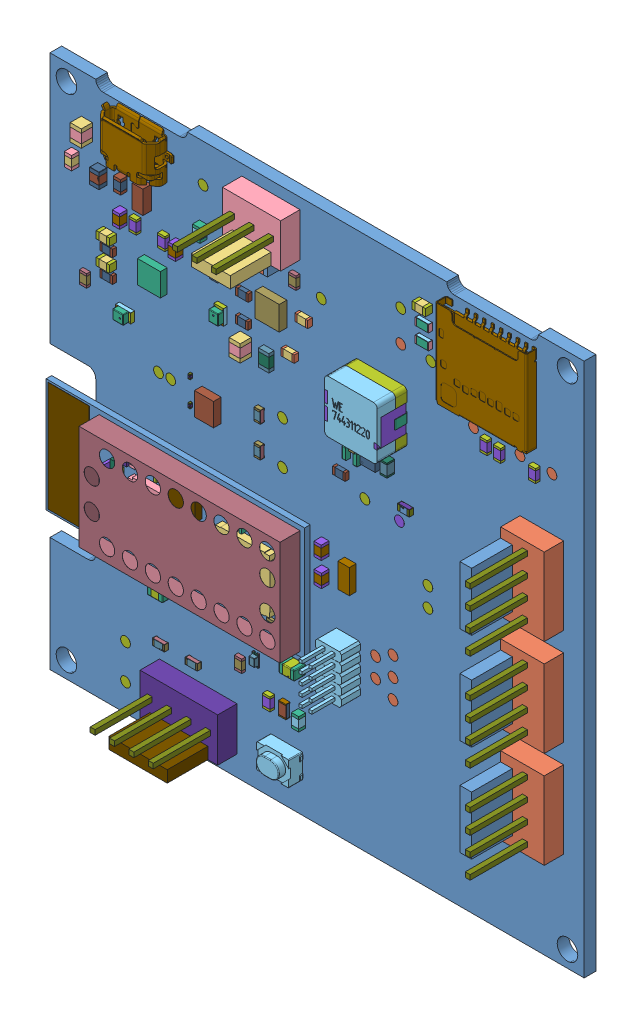
SolidWorks assembly IoTracking_PCB_new, configuration Default. Lengths in mm.
Overall size (70 70 13.59).
656 component instances, 214 part files, 0 mates.
Components (placement in the parent):
- IoTracking_PCB_new.step-1: IoTracking_PCB_new.step [Default] at origin size (70.02 70.02 13.59)
  - Board.step-1: Board.step [Default] at origin size (70 70 1.53)
    - Open CASCADE STEP translator 6.8 1.1.1.step-1: Open CASCADE STEP translator 6.8 1.1.1.step [Default] at (0 0 -1.5342) size (70 70 1.53)
  - TP8.step-1: TP8.step [Default] at origin size (1.27 1.27 0.02)
    - 6125959248.step-1: 6125959248.step [Default] at (42.672 22.86 -0.015) x (-1 0 0) z (0 0 1) size (1.27 1.27 0.02)
      - Cylinder.step-1: Cylinder.step [Default] at origin size (1.27 1.27 0.02)
  - C3.step-1: C3.step [Default] at origin size (0.95 1.75 0.95)
    - 6125953728.step-1: 6125953728.step [Default] at (3.302 59.817 0) size (0.95 0.95 0.95)
      - Extruded.step-1: Extruded.step [Default] at origin size (0.95 0.95 0.95)
    - 6125953568.step-1: 6125953568.step [Default] at (3.302 59.142 0) size (0.95 0.4 0.95)
      - Extruded-0.step-1: Extruded-0.step [Default] at origin size (0.95 0.4 0.95)
    - 6125953568.step-2: 6125953568.step [Default] at (3.302 60.492 0) size (0.95 0.4 0.95)
      - Extruded-0.step-1: Extruded-0.step [Default] at origin size (0.95 0.4 0.95)
  - B1.step-1: B1.step [Default] at origin size (4.6 3.2 2.5)
    - PTS810_CK_Switch.step-1: PTS810_CK_Switch.step [Default] at (30.9881 5.5881 0) x (1 0 0) z (0 -1 0) size (4.6 2.5 3.2)
  - C9.step-1: C9.step [Default] at origin size (2.01 1.25 1.52)
    - Cap_AVX_0805YA103FAT2A_eec.step-1: Cap_AVX_0805YA103FAT2A_eec.step [Default] at (32.512 16.764 0) x (1 0 0) z (0 0 1) size (2.01 1.25 1.52)
      - Terminals.step-1: Terminals.step [Default] at origin size (2.01 1.25 1.52)
      - Electrode.step-1: Electrode.step [Default] at origin size (1.01 1.25 1.52)
      - AVX.step-1: AVX.step [Default] at origin size (0.37 0.13 0)
  - X1.step-1: X1.step [Default] at origin size (1.5 3.2 0.9)
    - 6125955888.step-1: 6125955888.step [Default] at (39.37 30.48 0) size (1.5 3.2 0.9)
      - Extruded-1.step-1: Extruded-1.step [Default] at origin size (1.5 3.2 0.9)
  - U_Buck1.step-1: U_Buck1.step [Default] at origin size (2 2 0.8)
    - 5928732880.step-1: 5928732880.step [Default] at (42.418 45.466 0) x (0 1 0) z (1 0 0) size (2 0.8 2)
  - U_Accel1.step-1: U_Accel1.step [Default] at origin size (2.5 3 1)
    - 6125958608.step-1: 6125958608.step [Default] at (21.1836 40.64 0) size (2.5 3 1)
      - Extruded-2.step-1: Extruded-2.step [Default] at origin size (2.5 3 1)
  - U4.step-1: U4.step [Default] at origin size (3.15 3.15 1)
    - 6127423232.step-1: 6127423232.step [Default] at (29.464 55.88 0) size (3.15 3.15 1)
      - Extruded-3.step-1: Extruded-3.step [Default] at origin size (3.15 3.15 1)
  - U3.step-1: U3.step [Default] at origin size (33.86 14.91 3.4)
    - SAMW25.step-1: SAMW25.step [Default] at (60.2291 61.0334 0) x (1 0 0) z (0 0 1) size (33.86 14.91 3.4)
      - wifimodule.step-1: wifimodule.step [Default] at (-37.621 -27.6339 0) x (-1 0 0) z (0 0 1) size (26.34 13.71 2.64)
      - wifimodule_2.step-1: wifimodule_2.step [Default] at (-37.621 -27.6339 0) x (-1 0 0) z (0 0 1) size (0.33 0.95 0.33)
      - wifimodule_3.step-1: wifimodule_3.step [Default] at (-37.621 -27.6339 0) x (-1 0 0) z (0 0 1) size (0.95 0.33 0.33)
      - wifimodule_4.step-1: wifimodule_4.step [Default] at (-37.621 -27.6339 0) x (-1 0 0) z (0 0 1) size (0.33 0.95 0.33)
      - wifimodule_5.step-1: wifimodule_5.step [Default] at (-37.621 -27.6339 0) x (-1 0 0) z (0 0 1) size (0.33 0.95 0.33)
      - wifimodule_6.step-1: wifimodule_6.step [Default] at (-37.621 -27.6339 0) x (-1 0 0) z (0 0 1) size (0.33 0.95 0.33)
      - wifimodule_7.step-1: wifimodule_7.step [Default] at (-37.621 -27.6339 0) x (-1 0 0) z (0 0 1) size (3.7 2.1 0.6)
      - wifimodule_8.step-1: wifimodule_8.step [Default] at (-37.621 -27.6339 0) x (-1 0 0) z (0 0 1) size (0.33 0.95 0.33)
      - wifimodule_9.step-1: wifimodule_9.step [Default] at (-37.621 -27.6339 0) x (-1 0 0) z (0 0 1) size (0.5 1 0.03)
      - wifimodule_10.step-1: wifimodule_10.step [Default] at (-37.621 -27.6339 0) x (-1 0 0) z (0 0 1) size (0.5 1 0.03)
      - wifimodule_11.step-1: wifimodule_11.step [Default] at (-37.621 -27.6339 0) x (-1 0 0) z (0 0 1) size (0.5 1 0.03)
      - wifimodule_12.step-1: wifimodule_12.step [Default] at (-37.621 -27.6339 0) x (-1 0 0) z (0 0 1) size (0.5 1 0.03)
      - wifimodule_13.step-1: wifimodule_13.step [Default] at (-37.621 -27.6339 0) x (-1 0 0) z (0 0 1) size (0.5 1 0.03)
      - wifimodule_14.step-1: wifimodule_14.step [Default] at (-37.621 -27.6339 0) x (-1 0 0) z (0 0 1) size (0.5 1 0.03)
      - wifimodule_15.step-1: wifimodule_15.step [Default] at (-37.621 -27.6339 0) x (-1 0 0) z (0 0 1) size (0.5 1 0.03)
      - wifimodule_16.step-1: wifimodule_16.step [Default] at (-37.621 -27.6339 0) x (-1 0 0) z (0 0 1) size (0.5 1 0.03)
      - wifimodule_17.step-1: wifimodule_17.step [Default] at (-37.621 -27.6339 0) x (-1 0 0) z (0 0 1) size (0.5 1 0.03)
      - wifimodule_18.step-1: wifimodule_18.step [Default] at (-37.621 -27.6339 0) x (-1 0 0) z (0 0 1) size (0.5 1 0.03)
      - wifimodule_19.step-1: wifimodule_19.step [Default] at (-37.621 -27.6339 0) x (-1 0 0) z (0 0 1) size (0.5 1 0.03)
      - wifimodule_20.step-1: wifimodule_20.step [Default] at (-37.621 -27.6339 0) x (-1 0 0) z (0 0 1) size (0.5 1 0.03)
      - wifimodule_21.step-1: wifimodule_21.step [Default] at (-37.621 -27.6339 0) x (-1 0 0) z (0 0 1) size (0.5 1 0.03)
      - wifimodule_22.step-1: wifimodule_22.step [Default] at (-37.621 -27.6339 0) x (-1 0 0) z (0 0 1) size (0.5 1 0.03)
      - wifimodule_23.step-1: wifimodule_23.step [Default] at (-37.621 -27.6339 0) x (-1 0 0) z (0 0 1) size (0.5 1 0.03)
      - wifimodule_24.step-1: wifimodule_24.step [Default] at (-37.621 -27.6339 0) x (-1 0 0) z (0 0 1) size (0.95 0.33 0.33)
      - wifimodule_25.step-1: wifimodule_25.step [Default] at (-37.621 -27.6339 0) x (-1 0 0) z (0 0 1) size (0.95 0.33 0.33)
      - wifimodule_26.step-1: wifimodule_26.step [Default] at (-37.621 -27.6339 0) x (-1 0 0) z (0 0 1) size (0.95 0.33 0.33)
      - wifimodule_27.step-1: wifimodule_27.step [Default] at (-37.621 -27.6339 0) x (-1 0 0) z (0 0 1) size (0.33 0.95 0.33)
      - wifimodule_28.step-1: wifimodule_28.step [Default] at (-37.621 -27.6339 0) x (-1 0 0) z (0 0 1) size (0.95 0.33 0.33)
      - wifimodule_29.step-1: wifimodule_29.step [Default] at (-37.621 -27.6339 0) x (-1 0 0) z (0 0 1) size (0.33 0.95 0.33)
      - wifimodule_30.step-1: wifimodule_30.step [Default] at (-37.621 -27.6339 0) x (-1 0 0) z (0 0 1) size (0.95 0.33 0.33)
      - wifimodule_31.step-1: wifimodule_31.step [Default] at (-37.621 -27.6339 0) x (-1 0 0) z (0 0 1) size (0.33 0.95 0.33)
      - wifimodule_32.step-1: wifimodule_32.step [Default] at (-37.621 -27.6339 0) x (-1 0 0) z (0 0 1) size (0.33 0.74 1)
      - wifimodule_33.step-1: wifimodule_33.step [Default] at (-37.621 -27.6339 0) x (-1 0 0) z (0 0 1) size (0.74 0.33 1)
      - wifimodule_34.step-1: wifimodule_34.step [Default] at (-37.621 -27.6339 0) x (-1 0 0) z (0 0 1) size (2.68 1.78 1.04)
      - wifimodule_35.step-1: wifimodule_35.step [Default] at (-37.621 -27.6339 0) x (-1 0 0) z (0 0 1) size (1.56 1.02 0.66)
      - wifimodule_36.step-1: wifimodule_36.step [Default] at (-37.621 -27.6339 0) x (-1 0 0) z (0 0 1) size (0.91 2.06 0.41)
      - wifimodule_37.step-1: wifimodule_37.step [Default] at (-37.621 -27.6339 0) x (-1 0 0) z (0 0 1) size (2.06 0.91 0.41)
      - wifimodule_38.step-1: wifimodule_38.step [Default] at (-37.621 -27.6339 0) x (-1 0 0) z (0 0 1) size (2.06 0.91 0.41)
      - wifimodule_39.step-1: wifimodule_39.step [Default] at (-37.621 -27.6339 0) x (-1 0 0) z (0 0 1) size (0.91 2.06 0.41)
      - wifimodule_40.step-1: wifimodule_40.step [Default] at (-37.621 -27.6339 0) x (-1 0 0) z (0 0 1) size (0.33 0.74 1)
      - wifimodule_41.step-1: wifimodule_41.step [Default] at (-37.621 -27.6339 0) x (-1 0 0) z (0 0 1) size (0.33 0.74 1)
      - wifimodule_42.step-1: wifimodule_42.step [Default] at (-37.621 -27.6339 0) x (-1 0 0) z (0 0 1) size (0.33 0.74 1)
      - wifimodule_43.step-1: wifimodule_43.step [Default] at (-37.621 -27.6339 0) x (-1 0 0) z (0 0 1) size (0.33 0.74 1)
      - wifimodule_44.step-1: wifimodule_44.step [Default] at (-37.621 -27.6339 0) x (-1 0 0) z (0 0 1) size (0.33 0.74 1)
      - wifimodule_45.step-1: wifimodule_45.step [Default] at (-37.621 -27.6339 0) x (-1 0 0) z (0 0 1) size (0.74 0.33 1)
      - wifimodule_46.step-1: wifimodule_46.step [Default] at (-37.621 -27.6339 0) x (-1 0 0) z (0 0 1) size (0.74 0.33 1)
      - wifimodule_47.step-1: wifimodule_47.step [Default] at (-37.621 -27.6339 0) x (-1 0 0) z (0 0 1) size (0.33 0.74 1)
      - wifimodule_48.step-1: wifimodule_48.step [Default] at (-37.621 -27.6339 0) x (-1 0 0) z (0 0 1) size (0.33 0.74 1)
      - wifimodule_49.step-1: wifimodule_49.step [Default] at (-37.621 -27.6339 0) x (-1 0 0) z (0 0 1) size (0.33 0.74 1)
      - wifimodule_50.step-1: wifimodule_50.step [Default] at (-37.621 -27.6339 0) x (-1 0 0) z (0 0 1) size (0.74 0.33 1)
      - wifimodule_51.step-1: wifimodule_51.step [Default] at (-37.621 -27.6339 0) x (-1 0 0) z (0 0 1) size (0.74 0.33 1)
      - wifimodule_52.step-1: wifimodule_52.step [Default] at (-37.621 -27.6339 0) x (-1 0 0) z (0 0 1) size (0.74 0.33 1)
      - wifimodule_53.step-1: wifimodule_53.step [Default] at (-37.621 -27.6339 0) x (-1 0 0) z (0 0 1) size (0.74 0.33 1)
      - wifimodule_54.step-1: wifimodule_54.step [Default] at (-37.621 -27.6339 0) x (-1 0 0) z (0 0 1) size (0.74 0.33 1)
      - wifimodule_55.step-1: wifimodule_55.step [Default] at (-37.621 -27.6339 0) x (-1 0 0) z (0 0 1) size (0.33 0.74 1)
      - wifimodule_56.step-1: wifimodule_56.step [Default] at (-37.621 -27.6339 0) x (-1 0 0) z (0 0 1) size (0.74 0.33 1)
      - wifimodule_57.step-1: wifimodule_57.step [Default] at (-37.621 -27.6339 0) x (-1 0 0) z (0 0 1) size (0.42 1.12 0.33)
      - wifimodule_58.step-1: wifimodule_58.step [Default] at (-37.621 -27.6339 0) x (-1 0 0) z (0 0 1) size (0.5 1 0.03)
      - wifimodule_59.step-1: wifimodule_59.step [Default] at (-37.621 -27.6339 0) x (-1 0 0) z (0 0 1) size (0.42 1.12 0.33)
      - wifimodule_60.step-1: wifimodule_60.step [Default] at (-37.621 -27.6339 0) x (-1 0 0) z (0 0 1) size (3.66 4.34 0.91)
      - wifimodule_61.step-1: wifimodule_61.step [Default] at (-37.621 -27.6339 0) x (-1 0 0) z (0 0 1) size (0.5 1 0.03)
      - wifimodule_62.step-1: wifimodule_62.step [Default] at (-37.621 -27.6339 0) x (-1 0 0) z (0 0 1) size (0.5 1 0.03)
      - wifimodule_63.step-1: wifimodule_63.step [Default] at (-37.621 -27.6339 0) x (-1 0 0) z (0 0 1) size (0.5 1 0.03)
      - wifimodule_64.step-1: wifimodule_64.step [Default] at (-37.621 -27.6339 0) x (-1 0 0) z (0 0 1) size (0.5 1 0.03)
      - wifimodule_65.step-1: wifimodule_65.step [Default] at (-37.621 -27.6339 0) x (-1 0 0) z (0 0 1) size (1 0.5 0.03)
      - wifimodule_66.step-1: wifimodule_66.step [Default] at (-37.621 -27.6339 0) x (-1 0 0) z (0 0 1) size (1 0.5 0.03)
      - wifimodule_67.step-1: wifimodule_67.step [Default] at (-37.621 -27.6339 0) x (-1 0 0) z (0 0 1) size (1 0.5 0.03)
      - wifimodule_68.step-1: wifimodule_68.step [Default] at (-37.621 -27.6339 0) x (-1 0 0) z (0 0 1) size (1 0.5 0.03)
      - wifimodule_69.step-1: wifimodule_69.step [Default] at (-37.621 -27.6339 0) x (-1 0 0) z (0 0 1) size (1 0.5 0.03)
      - wifimodule_70.step-1: wifimodule_70.step [Default] at (-37.621 -27.6339 0) x (-1 0 0) z (0 0 1) size (1 0.5 0.03)
      - wifimodule_71.step-1: wifimodule_71.step [Default] at (-37.621 -27.6339 0) x (-1 0 0) z (0 0 1) size (1 0.5 0.03)
      - wifimodule_72.step-1: wifimodule_72.step [Default] at (-37.621 -27.6339 0) x (-1 0 0) z (0 0 1) size (0.5 1 0.03)
      - wifimodule_73.step-1: wifimodule_73.step [Default] at (-37.621 -27.6339 0) x (-1 0 0) z (0 0 1) size (0.5 1 0.03)
      - wifimodule_74.step-1: wifimodule_74.step [Default] at (-37.621 -27.6339 0) x (-1 0 0) z (0 0 1) size (0.5 1 0.03)
      - wifimodule_75.step-1: wifimodule_75.step [Default] at (-37.621 -27.6339 0) x (-1 0 0) z (0 0 1) size (0.5 1 0.03)
      - wifimodule_76.step-1: wifimodule_76.step [Default] at (-37.621 -27.6339 0) x (-1 0 0) z (0 0 1) size (0.5 1 0.03)
      - wifimodule_77.step-1: wifimodule_77.step [Default] at (-37.621 -27.6339 0) x (-1 0 0) z (0 0 1) size (0.5 1 0.03)
      - wifimodule_78.step-1: wifimodule_78.step [Default] at (-37.621 -27.6339 0) x (-1 0 0) z (0 0 1) size (0.5 1 0.03)
      - wifimodule_79.step-1: wifimodule_79.step [Default] at (-37.621 -27.6339 0) x (-1 0 0) z (0 0 1) size (0.5 1 0.03)
      - wifimodule_80.step-1: wifimodule_80.step [Default] at (-37.621 -27.6339 0) x (-1 0 0) z (0 0 1) size (0.95 0.33 0.33)
      - wifimodule_81.step-1: wifimodule_81.step [Default] at (-37.621 -27.6339 0) x (-1 0 0) z (0 0 1) size (0.95 0.33 0.33)
      - wifimodule_82.step-1: wifimodule_82.step [Default] at (-37.621 -27.6339 0) x (-1 0 0) z (0 0 1) size (0.33 0.95 0.33)
      - wifimodule_83.step-1: wifimodule_83.step [Default] at (-37.621 -27.6339 0) x (-1 0 0) z (0 0 1) size (0.33 0.95 0.33)
      - wifimodule_84.step-1: wifimodule_84.step [Default] at (-37.621 -27.6339 0) x (-1 0 0) z (0 0 1) size (1.12 0.42 0.33)
      - wifimodule_85.step-1: wifimodule_85.step [Default] at (-37.621 -27.6339 0) x (-1 0 0) z (0 0 1) size (0.95 0.33 0.33)
      - wifimodule_86.step-1: wifimodule_86.step [Default] at (-37.621 -27.6339 0) x (-1 0 0) z (0 0 1) size (0.42 1.12 0.33)
      - wifimodule_87.step-1: wifimodule_87.step [Default] at (-37.621 -27.6339 0) x (-1 0 0) z (0 0 1) size (0.95 0.33 0.33)
      - wifimodule_88.step-1: wifimodule_88.step [Default] at (-37.621 -27.6339 0) x (-1 0 0) z (0 0 1) size (1 0.5 0.03)
      - wifimodule_89.step-1: wifimodule_89.step [Default] at (-37.621 -27.6339 0) x (-1 0 0) z (0 0 1) size (0.5 1 0.03)
      - wifimodule_90.step-1: wifimodule_90.step [Default] at (-37.621 -27.6339 0) x (-1 0 0) z (0 0 1) size (0.5 1 0.03)
      - wifimodule_91.step-1: wifimodule_91.step [Default] at (-37.621 -27.6339 0) x (-1 0 0) z (0 0 1) size (0.5 1 0.03)
      - wifimodule_92.step-1: wifimodule_92.step [Default] at (-37.621 -27.6339 0) x (-1 0 0) z (0 0 1) size (1 0.5 0.03)
      - wifimodule_93.step-1: wifimodule_93.step [Default] at (-37.621 -27.6339 0) x (-1 0 0) z (0 0 1) size (0.5 1 0.03)
      - wifimodule_94.step-1: wifimodule_94.step [Default] at (-37.621 -27.6339 0) x (-1 0 0) z (0 0 1) size (0.5 1 0.03)
      - wifimodule_95.step-1: wifimodule_95.step [Default] at (-37.621 -27.6339 0) x (-1 0 0) z (0 0 1) size (0.5 1 0.03)
      - wifimodule_96.step-1: wifimodule_96.step [Default] at (-37.621 -27.6339 0) x (-1 0 0) z (0 0 1) size (0.5 1 0.03)
      - wifimodule_97.step-1: wifimodule_97.step [Default] at (-37.621 -27.6339 0) x (-1 0 0) z (0 0 1) size (0.5 1 0.03)
      - wifimodule_98.step-1: wifimodule_98.step [Default] at (-37.621 -27.6339 0) x (-1 0 0) z (0 0 1) size (1 0.5 0.03)
      - wifimodule_99.step-1: wifimodule_99.step [Default] at (-37.621 -27.6339 0) x (-1 0 0) z (0 0 1) size (1 0.5 0.03)
      - wifimodule_100.step-1: wifimodule_100.step [Default] at (-37.621 -27.6339 0) x (-1 0 0) z (0 0 1) size (0.5 1 0.03)
      - wifimodule_101.step-1: wifimodule_101.step [Default] at (-37.621 -27.6339 0) x (-1 0 0) z (0 0 1) size (0.5 1 0.03)
      - wifimodule_102.step-1: wifimodule_102.step [Default] at (-37.621 -27.6339 0) x (-1 0 0) z (0 0 1) size (0.5 1 0.03)
      - wifimodule_103.step-1: wifimodule_103.step [Default] at (-37.621 -27.6339 0) x (-1 0 0) z (0 0 1) size (0.5 1 0.03)
      - wifimodule_104.step-1: wifimodule_104.step [Default] at (-37.621 -27.6339 0) x (-1 0 0) z (0 0 1) size (0.33 0.95 0.33)
      - wifimodule_105.step-1: wifimodule_105.step [Default] at (-37.621 -27.6339 0) x (-1 0 0) z (0 0 1) size (0.33 0.95 0.33)
      - wifimodule_106.step-1: wifimodule_106.step [Default] at (-37.621 -27.6339 0) x (-1 0 0) z (0 0 1) size (0.33 0.95 0.33)
      - wifimodule_107.step-1: wifimodule_107.step [Default] at (-37.621 -27.6339 0) x (-1 0 0) z (0 0 1) size (0.33 0.95 0.33)
      - wifimodule_108.step-1: wifimodule_108.step [Default] at (-37.621 -27.6339 0) x (-1 0 0) z (0 0 1) size (0.95 0.33 0.33)
      - wifimodule_109.step-1: wifimodule_109.step [Default] at (-37.621 -27.6339 0) x (-1 0 0) z (0 0 1) size (0.33 0.95 0.33)
      - wifimodule_110.step-1: wifimodule_110.step [Default] at (-37.621 -27.6339 0) x (-1 0 0) z (0 0 1) size (0.33 0.95 0.33)
      - wifimodule_111.step-1: wifimodule_111.step [Default] at (-37.621 -27.6339 0) x (-1 0 0) z (0 0 1) size (0.74 0.33 1)
      - wifimodule_112.step-1: wifimodule_112.step [Default] at (-37.621 -27.6339 0) x (-1 0 0) z (0 0 1) size (0.91 2.06 0.41)
      - wifimodule_113.step-1: wifimodule_113.step [Default] at (-37.621 -27.6339 0) x (-1 0 0) z (0 0 1) size (0.89 0.89 0.03)
      - wifimodule_114.step-1: wifimodule_114.step [Default] at (-37.621 -27.6339 0) x (-1 0 0) z (0 0 1) size (5.4 14.4 0.03)
      - wifimodule_115.step-1: wifimodule_115.step [Default] at (-37.621 -27.6339 0) x (-1 0 0) z (0 0 1) size (33.86 14.91 0.73)
      - wifimodule_116.step-1: wifimodule_116.step [Default] at (-37.621 -27.6339 0) x (-1 0 0) z (0 0 1) size (2.5 2.2 1.1)
      - wifimodule_117.step-1: wifimodule_117.step [Default] at (-37.621 -27.6339 0) x (-1 0 0) z (0 0 1) size (7.2 7.2 0.9)
      - wifimodule_118.step-1: wifimodule_118.step [Default] at (-37.621 -27.6339 0) x (-1 0 0) z (0 0 1) size (5.6 5.6 0.85)
  - U2.step-1: U2.step [Default] at origin size (3.4 6.35 7.85)
    - 10posheader.step-1: 10posheader.step [Default] at (38.989 22.86 0) x (0 -1 0) z (-1 0 0) size (6.35 7.85 3.4)
  - U1.step-1: U1.step [Default] at origin size (3 3 0.9)
    - 6127410672.step-1: 6127410672.step [Default] at (13.8684 51.7906 0) size (3 3 0.9)
      - Extruded-4.step-1: Extruded-4.step [Default] at origin size (3 3 0.9)
  - TP_OLED_2.step-1: TP_OLED_2.step [Default] at origin size (1.27 1.27 0.02)
    - 6127428272.step-1: 6127428272.step [Default] at (9.906 8.128 -0.015) x (0 1 0) z (0 0 1) size (1.27 1.27 0.02)
      - Cylinder-5.step-1: Cylinder-5.step [Default] at origin size (1.27 1.27 0.02)
  - TP_OLED_1.step-1: TP_OLED_1.step [Default] at origin size (1.27 1.27 0.02)
    - 6127428272.step-1: 6127428272.step [Default] at (9.906 3.556 -0.015) x (0 1 0) z (0 0 1) size (1.27 1.27 0.02)
      - Cylinder-5.step-1: Cylinder-5.step [Default] at origin size (1.27 1.27 0.02)
  - TP_GPS_2.step-1: TP_GPS_2.step [Default] at origin size (1.27 1.27 0.02)
    - 6127428272.step-1: 6127428272.step [Default] at (49.53 34.29 -0.015) x (0 1 0) z (0 0 1) size (1.27 1.27 0.02)
      - Cylinder-5.step-1: Cylinder-5.step [Default] at origin size (1.27 1.27 0.02)
  - TP_GPS_1.step-1: TP_GPS_1.step [Default] at origin size (1.27 1.27 0.02)
    - 6127428272.step-1: 6127428272.step [Default] at (49.53 31.75 -0.015) x (0 1 0) z (0 0 1) size (1.27 1.27 0.02)
      - Cylinder-5.step-1: Cylinder-5.step [Default] at origin size (1.27 1.27 0.02)
  - TP_BUCK_2.step-1: TP_BUCK_2.step [Default] at origin size (1.27 1.27 0.02)
    - 6127428272.step-1: 6127428272.step [Default] at (41.275 40.005 -0.015) x (0 1 0) z (0 0 1) size (1.27 1.27 0.02)
      - Cylinder-5.step-1: Cylinder-5.step [Default] at origin size (1.27 1.27 0.02)
  - TP_BUCK_1.step-1: TP_BUCK_1.step [Default] at origin size (1.27 1.27 0.02)
    - 6126688688.step-1: 6126688688.step [Default] at (45.7962 39.751 -0.015) x (1 0 0) z (0 0 1) size (1.27 1.27 0.02)
      - Cylinder-6.step-1: Cylinder-6.step [Default] at origin size (1.27 1.27 0.02)
  - TP_ACC_2.step-1: TP_ACC_2.step [Default] at origin size (1.27 1.27 0.02)
    - 6127428272.step-1: 6127428272.step [Default] at (30.48 43.815 -0.015) x (0 1 0) z (0 0 1) size (1.27 1.27 0.02)
      - Cylinder-5.step-1: Cylinder-5.step [Default] at origin size (1.27 1.27 0.02)
  - TP_ACC_1.step-1: TP_ACC_1.step [Default] at origin size (1.27 1.27 0.02)
    - 6127428272.step-1: 6127428272.step [Default] at (30.48 38.1762 -0.015) x (0 1 0) z (0 0 1) size (1.27 1.27 0.02)
      - Cylinder-5.step-1: Cylinder-5.step [Default] at origin size (1.27 1.27 0.02)
  - TP16.step-1: TP16.step [Default] at origin size (1.27 1.27 0.02)
    - 6125959248.step-1: 6125959248.step [Default] at (45.974 59.944 -0.015) x (-1 0 0) z (0 0 1) size (1.27 1.27 0.02)
      - Cylinder.step-1: Cylinder.step [Default] at origin size (1.27 1.27 0.02)
  - TP15.step-1: TP15.step [Default] at origin size (1.27 1.27 0.02)
    - 6125959248.step-1: 6125959248.step [Default] at (61.595 55.118 -0.015) x (-1 0 0) z (0 0 1) size (1.27 1.27 0.02)
      - Cylinder.step-1: Cylinder.step [Default] at origin size (1.27 1.27 0.02)
  - TP14.step-1: TP14.step [Default] at origin size (1.27 1.27 0.02)
    - 6125959248.step-1: 6125959248.step [Default] at (65.786 55.118 -0.015) x (-1 0 0) z (0 0 1) size (1.27 1.27 0.02)
      - Cylinder.step-1: Cylinder.step [Default] at origin size (1.27 1.27 0.02)
  - TP13.step-1: TP13.step [Default] at origin size (1.27 1.27 0.02)
    - 6125959248.step-1: 6125959248.step [Default] at (55.499 55.245 -0.015) x (-1 0 0) z (0 0 1) size (1.27 1.27 0.02)
      - Cylinder.step-1: Cylinder.step [Default] at origin size (1.27 1.27 0.02)
  - TP12.step-1: TP12.step [Default] at origin size (1.27 1.27 0.02)
    - 6127428272.step-1: 6127428272.step [Default] at (49.911 59.944 -0.015) x (0 1 0) z (0 0 1) size (1.27 1.27 0.02)
      - Cylinder-5.step-1: Cylinder-5.step [Default] at origin size (1.27 1.27 0.02)
  - TP11.step-1: TP11.step [Default] at origin size (1.27 1.27 0.02)
    - 6127428272.step-1: 6127428272.step [Default] at (45.974 64.008 -0.015) x (0 1 0) z (0 0 1) size (1.27 1.27 0.02)
      - Cylinder-5.step-1: Cylinder-5.step [Default] at origin size (1.27 1.27 0.02)
  - TP10.step-1: TP10.step [Default] at origin size (1.27 1.27 0.02)
    - 6125959248.step-1: 6125959248.step [Default] at (44.958 19.05 -0.015) x (-1 0 0) z (0 0 1) size (1.27 1.27 0.02)
      - Cylinder.step-1: Cylinder.step [Default] at origin size (1.27 1.27 0.02)
  - TP9.step-1: TP9.step [Default] at origin size (1.27 1.27 0.02)
    - 6125959248.step-1: 6125959248.step [Default] at (44.958 21.59 -0.015) x (-1 0 0) z (0 0 1) size (1.27 1.27 0.02)
      - Cylinder.step-1: Cylinder.step [Default] at origin size (1.27 1.27 0.02)
  - TP7.step-1: TP7.step [Default] at origin size (1.27 1.27 0.02)
    - 6125959248.step-1: 6125959248.step [Default] at (42.672 20.32 -0.015) x (-1 0 0) z (0 0 1) size (1.27 1.27 0.02)
      - Cylinder.step-1: Cylinder.step [Default] at origin size (1.27 1.27 0.02)
  - TP6.step-1: TP6.step [Default] at origin size (1.27 1.27 0.02)
    - 6125959248.step-1: 6125959248.step [Default] at (44.958 24.13 -0.015) x (-1 0 0) z (0 0 1) size (1.27 1.27 0.02)
      - Cylinder.step-1: Cylinder.step [Default] at origin size (1.27 1.27 0.02)
  - TP5.step-1: TP5.step [Default] at origin size (1.27 1.27 0.02)
    - 6127428272.step-1: 6127428272.step [Default] at (35.56 59.8932 -0.015) x (0 1 0) z (0 0 1) size (1.27 1.27 0.02)
      - Cylinder-5.step-1: Cylinder-5.step [Default] at origin size (1.27 1.27 0.02)
  - TP4.step-1: TP4.step [Default] at origin size (1.27 1.27 0.02)
    - 6127428272.step-1: 6127428272.step [Default] at (14.224 40.8444 -0.015) x (0 1 0) z (0 0 1) size (1.27 1.27 0.02)
      - Cylinder-5.step-1: Cylinder-5.step [Default] at origin size (1.27 1.27 0.02)
  - TP3.step-1: TP3.step [Default] at origin size (1.27 1.27 0.02)
    - 6127428272.step-1: 6127428272.step [Default] at (19.8882 16.51 -0.015) x (0 1 0) z (0 0 1) size (1.27 1.27 0.02)
      - Cylinder-5.step-1: Cylinder-5.step [Default] at origin size (1.27 1.27 0.02)
  - TP2.step-1: TP2.step [Default] at origin size (1.27 1.27 0.02)
    - 6127428272.step-1: 6127428272.step [Default] at (15.8242 40.8686 -0.015) x (0 1 0) z (0 0 1) size (1.27 1.27 0.02)
      - Cylinder-5.step-1: Cylinder-5.step [Default] at origin size (1.27 1.27 0.02)
  - TP1.step-1: TP1.step [Default] at origin size (1.27 1.27 0.02)
    - 6127428272.step-1: 6127428272.step [Default] at (20.066 65.024 -0.015) x (0 1 0) z (0 0 1) size (1.27 1.27 0.02)
      - Cylinder-5.step-1: Cylinder-5.step [Default] at origin size (1.27 1.27 0.02)
  - SD1.step-1: SD1.step [Default] at origin size (11.95 11.4 1.45)
    - 1040310811.step-1: 1040310811.step [Default] at (102.3746 60.988 0.61) x (-1 0 0) z (0 0 1) size (11.95 11.4 1.45)
      - Open CASCADE STEP translator 6.8 1.36.1.1.step-1: Open CASCADE STEP translator 6.8 1.36.1.1.step [Default] at origin size (11.95 11.4 1.45)
      - Open CASCADE STEP translator 6.8 1.36.1.2.step-1: Open CASCADE STEP translator 6.8 1.36.1.2.step [Default] at origin
  - RJ1.step-1: RJ1.step [Default] at origin size (1.65 0.95 0.5)
    - 6125952048.step-1: 6125952048.step [Default] at (38.354 41.656 0) size (1.05 0.95 0.5)
      - Extruded-7.step-1: Extruded-7.step [Default] at origin size (1.05 0.95 0.5)
    - 6125951888.step-1: 6125951888.step [Default] at (37.679 41.656 0) size (0.3 0.95 0.5)
      - Extruded-8.step-1: Extruded-8.step [Default] at origin size (0.3 0.95 0.5)
    - 6125951888.step-2: 6125951888.step [Default] at (39.029 41.656 0) size (0.3 0.95 0.5)
      - Extruded-8.step-1: Extruded-8.step [Default] at origin size (0.3 0.95 0.5)
  - R_O2.step-1: R_O2.step [Default] at origin size (1.6 0.8 0.55)
    - Res_Yageo_AT0603CRD0711R5L_eec.step-1: Res_Yageo_AT0603CRD0711R5L_eec.step [Default] at (19.05 10.414 0) x (-1 0 0) z (0 0 1) size (1.6 0.8 0.55)
      - 2.step-1: 2.step [Default] at origin size (1.6 0.8 0.55)
        - Open CASCADE STEP translator 6.8 1.38.1.1.1.step-1: Open CASCADE STEP translator 6.8 1.38.1.1.1.step [Default] at origin size (1.6 0.8 0.55)
        - Open CASCADE STEP translator 6.8 1.38.1.1.2.step-1: Open CASCADE STEP translator 6.8 1.38.1.1.2.step [Default] at origin
      - 3.step-1: 3.step [Default] at origin size (1.5 0.8 0.45)
        - Open CASCADE STEP translator 6.8 1.38.1.2.1.step-1: Open CASCADE STEP translator 6.8 1.38.1.2.1.step [Default] at origin size (1.5 0.8 0.45)
        - Open CASCADE STEP translator 6.8 1.38.1.2.2.step-1: Open CASCADE STEP translator 6.8 1.38.1.2.2.step [Default] at origin
      - 4.step-1: 4.step [Default] at origin size (1.2 0.8 0.05)
        - Open CASCADE STEP translator 6.8 1.38.1.3.1.step-1: Open CASCADE STEP translator 6.8 1.38.1.3.1.step [Default] at origin size (1.2 0.8 0.05)
        - Open CASCADE STEP translator 6.8 1.38.1.3.2.step-1: Open CASCADE STEP translator 6.8 1.38.1.3.2.step [Default] at origin
      - 5.step-1: 5.step [Default] at (-0.0114 0.0028 0.4505) size (0.29 0.05 0.11)
  - R_O1.step-1: R_O1.step [Default] at origin size (1.6 0.8 0.55)
    - Res_Yageo_AT0603CRD0711R5L_eec.step-1: Res_Yageo_AT0603CRD0711R5L_eec.step [Default] at (14.732 10.414 0) x (1 0 0) z (0 0 1) size (1.6 0.8 0.55)
      - 2.step-1: 2.step [Default] at origin size (1.6 0.8 0.55)
        - Open CASCADE STEP translator 6.8 1.38.1.1.1.step-1: Open CASCADE STEP translator 6.8 1.38.1.1.1.step [Default] at origin size (1.6 0.8 0.55)
        - Open CASCADE STEP translator 6.8 1.38.1.1.2.step-1: Open CASCADE STEP translator 6.8 1.38.1.1.2.step [Default] at origin
      - 3.step-1: 3.step [Default] at origin size (1.5 0.8 0.45)
        - Open CASCADE STEP translator 6.8 1.38.1.2.1.step-1: Open CASCADE STEP translator 6.8 1.38.1.2.1.step [Default] at origin size (1.5 0.8 0.45)
        - Open CASCADE STEP translator 6.8 1.38.1.2.2.step-1: Open CASCADE STEP translator 6.8 1.38.1.2.2.step [Default] at origin
      - 4.step-1: 4.step [Default] at origin size (1.2 0.8 0.05)
        - Open CASCADE STEP translator 6.8 1.38.1.3.1.step-1: Open CASCADE STEP translator 6.8 1.38.1.3.1.step [Default] at origin size (1.2 0.8 0.05)
        - Open CASCADE STEP translator 6.8 1.38.1.3.2.step-1: Open CASCADE STEP translator 6.8 1.38.1.3.2.step [Default] at origin
      - 5.step-1: 5.step [Default] at (-0.0114 0.0028 0.4505) size (0.29 0.05 0.11)
  - R_B1.step-1: R_B1.step [Default] at origin size (1.55 0.8 0.56)
    - Res_TE_Connectivity_CPF0603B2K55E1_eec.step-1: Res_TE_Connectivity_CPF0603B2K55E1_eec.step [Default] at (46.863 41.783 0) x (1 0 0) z (0 0 1) size (1.55 0.8 0.56)
      - 1.step-1: 1.step [Default] at origin size (1.55 0.8 0.55)
      - 2-9.step-1: 2-9.step [Default] at origin size (1.45 0.8 0.5)
      - TE_connectivity_Logo_1.step-1: TE_connectivity_Logo_1.step [Default] at (5.0457 3.7568 0.451) x (-1 0 0) z (0 0 1) size (0.47 0.17 0.11)
      - 3-10.step-1: 3-10.step [Default] at origin size (0.95 0.8 0.05)
  - R_A2.step-1: R_A2.step [Default] at origin size (0.8 1.6 0.55)
    - Res_Yageo_AT0603CRD0711R5L_eec.step-1: Res_Yageo_AT0603CRD0711R5L_eec.step [Default] at (27.686 42.926 0) x (0 -1 0) z (0 0 1) size (1.6 0.8 0.55)
      - 2.step-1: 2.step [Default] at origin size (1.6 0.8 0.55)
        - Open CASCADE STEP translator 6.8 1.38.1.1.1.step-1: Open CASCADE STEP translator 6.8 1.38.1.1.1.step [Default] at origin size (1.6 0.8 0.55)
        - Open CASCADE STEP translator 6.8 1.38.1.1.2.step-1: Open CASCADE STEP translator 6.8 1.38.1.1.2.step [Default] at origin
      - 3.step-1: 3.step [Default] at origin size (1.5 0.8 0.45)
        - Open CASCADE STEP translator 6.8 1.38.1.2.1.step-1: Open CASCADE STEP translator 6.8 1.38.1.2.1.step [Default] at origin size (1.5 0.8 0.45)
        - Open CASCADE STEP translator 6.8 1.38.1.2.2.step-1: Open CASCADE STEP translator 6.8 1.38.1.2.2.step [Default] at origin
      - 4.step-1: 4.step [Default] at origin size (1.2 0.8 0.05)
        - Open CASCADE STEP translator 6.8 1.38.1.3.1.step-1: Open CASCADE STEP translator 6.8 1.38.1.3.1.step [Default] at origin size (1.2 0.8 0.05)
        - Open CASCADE STEP translator 6.8 1.38.1.3.2.step-1: Open CASCADE STEP translator 6.8 1.38.1.3.2.step [Default] at origin
      - 5.step-1: 5.step [Default] at (-0.0114 0.0028 0.4505) size (0.29 0.05 0.11)
  - R_A1.step-1: R_A1.step [Default] at origin size (0.8 1.6 0.55)
    - Res_Yageo_AT0603CRD0711R5L_eec.step-1: Res_Yageo_AT0603CRD0711R5L_eec.step [Default] at (27.686 38.862 0) x (0 1 0) z (0 0 1) size (1.6 0.8 0.55)
      - 2.step-1: 2.step [Default] at origin size (1.6 0.8 0.55)
        - Open CASCADE STEP translator 6.8 1.38.1.1.1.step-1: Open CASCADE STEP translator 6.8 1.38.1.1.1.step [Default] at origin size (1.6 0.8 0.55)
        - Open CASCADE STEP translator 6.8 1.38.1.1.2.step-1: Open CASCADE STEP translator 6.8 1.38.1.1.2.step [Default] at origin
      - 3.step-1: 3.step [Default] at origin size (1.5 0.8 0.45)
        - Open CASCADE STEP translator 6.8 1.38.1.2.1.step-1: Open CASCADE STEP translator 6.8 1.38.1.2.1.step [Default] at origin size (1.5 0.8 0.45)
        - Open CASCADE STEP translator 6.8 1.38.1.2.2.step-1: Open CASCADE STEP translator 6.8 1.38.1.2.2.step [Default] at origin
      - 4.step-1: 4.step [Default] at origin size (1.2 0.8 0.05)
        - Open CASCADE STEP translator 6.8 1.38.1.3.1.step-1: Open CASCADE STEP translator 6.8 1.38.1.3.1.step [Default] at origin size (1.2 0.8 0.05)
        - Open CASCADE STEP translator 6.8 1.38.1.3.2.step-1: Open CASCADE STEP translator 6.8 1.38.1.3.2.step [Default] at origin
      - 5.step-1: 5.step [Default] at (-0.0114 0.0028 0.4505) size (0.29 0.05 0.11)
  - R19.step-1: R19.step [Default] at origin size (1.7 0.95 0.6)
    - 6127424752.step-1: 6127424752.step [Default] at (32.8129 56.6419 0) size (0.27 0.95 0.6)
      - Extruded-11.step-1: Extruded-11.step [Default] at origin size (0.27 0.95 0.6)
    - 6127424592.step-1: 6127424592.step [Default] at (33.5279 56.6419 0) size (1.16 0.95 0.6)
      - Extruded-12.step-1: Extruded-12.step [Default] at origin size (1.16 0.95 0.6)
    - 6127424752.step-2: 6127424752.step [Default] at (34.2429 56.6419 0) size (0.27 0.95 0.6)
      - Extruded-11.step-1: Extruded-11.step [Default] at origin size (0.27 0.95 0.6)
  - R18.step-1: R18.step [Default] at origin size (1.7 0.95 0.6)
    - 6127424752.step-1: 6127424752.step [Default] at (31.0349 51.8159 0) size (0.27 0.95 0.6)
      - Extruded-11.step-1: Extruded-11.step [Default] at origin size (0.27 0.95 0.6)
    - 6127424592.step-1: 6127424592.step [Default] at (31.7499 51.8159 0) size (1.16 0.95 0.6)
      - Extruded-12.step-1: Extruded-12.step [Default] at origin size (1.16 0.95 0.6)
    - 6127424752.step-2: 6127424752.step [Default] at (32.4649 51.8159 0) size (0.27 0.95 0.6)
      - Extruded-11.step-1: Extruded-11.step [Default] at origin size (0.27 0.95 0.6)
  - R17.step-1: R17.step [Default] at origin size (1.65 0.95 0.5)
    - 6125951888.step-1: 6125951888.step [Default] at (24.979 55.626 0) size (0.3 0.95 0.5)
      - Extruded-8.step-1: Extruded-8.step [Default] at origin size (0.3 0.95 0.5)
    - 6125951888.step-2: 6125951888.step [Default] at (26.329 55.626 0) size (0.3 0.95 0.5)
      - Extruded-8.step-1: Extruded-8.step [Default] at origin size (0.3 0.95 0.5)
    - 6125952048.step-1: 6125952048.step [Default] at (25.654 55.626 0) size (1.05 0.95 0.5)
      - Extruded-7.step-1: Extruded-7.step [Default] at origin size (1.05 0.95 0.5)
  - R16.step-1: R16.step [Default] at origin size (1.65 0.95 0.5)
    - 6125951888.step-1: 6125951888.step [Default] at (24.9374 52.4256 0) size (0.3 0.95 0.5)
      - Extruded-8.step-1: Extruded-8.step [Default] at origin size (0.3 0.95 0.5)
    - 6125951888.step-2: 6125951888.step [Default] at (26.2874 52.4256 0) size (0.3 0.95 0.5)
      - Extruded-8.step-1: Extruded-8.step [Default] at origin size (0.3 0.95 0.5)
    - 6125952048.step-1: 6125952048.step [Default] at (25.6124 52.4256 0) size (1.05 0.95 0.5)
      - Extruded-7.step-1: Extruded-7.step [Default] at origin size (1.05 0.95 0.5)
  - R15.step-1: R15.step [Default] at origin size (1.75 0.95 0.55)
    - 5928733040.step-1: 5928733040.step [Default] at (49.276 61.976 0) x (-1 0 0) z (0 0 1) size (1.75 0.95 0.55)
      - Terminal.step-1: Terminal.step [Default] at (-0.875 -0.475 0) size (0.15 0.95 0.55)
        - Open_CASCADE_STEP_translator_6.8_1.2.1.step-1: Open_CASCADE_STEP_translator_6.8_1.2.1.step [Default] at origin size (0.15 0.95 0.55)
      - Terminal.step-2: Terminal.step [Default] at (0.875 0.475 0) x (-1 0 0) z (0 0 1) size (0.15 0.95 0.55)
        - Open_CASCADE_STEP_translator_6.8_1.2.1.step-1: Open_CASCADE_STEP_translator_6.8_1.2.1.step [Default] at origin size (0.15 0.95 0.55)
      - Mid_Body.step-1: Mid_Body.step [Default] at (-0.875 -0.475 0) size (1.64 0.95 0.44)
      - Mark.step-1: Mark.step [Default] at (-0.725 -0.475 0.495) size (1.45 0.95 0.06)
  - R14.step-1: R14.step [Default] at origin size (1.75 0.95 0.55)
    - 5928733040.step-1: 5928733040.step [Default] at (49.276 64.008 0) x (-1 0 0) z (0 0 1) size (1.75 0.95 0.55)
      - Terminal.step-1: Terminal.step [Default] at (-0.875 -0.475 0) size (0.15 0.95 0.55)
        - Open_CASCADE_STEP_translator_6.8_1.2.1.step-1: Open_CASCADE_STEP_translator_6.8_1.2.1.step [Default] at origin size (0.15 0.95 0.55)
      - Terminal.step-2: Terminal.step [Default] at (0.875 0.475 0) x (-1 0 0) z (0 0 1) size (0.15 0.95 0.55)
        - Open_CASCADE_STEP_translator_6.8_1.2.1.step-1: Open_CASCADE_STEP_translator_6.8_1.2.1.step [Default] at origin size (0.15 0.95 0.55)
      - Mid_Body.step-1: Mid_Body.step [Default] at (-0.875 -0.475 0) size (1.64 0.95 0.44)
      - Mark.step-1: Mark.step [Default] at (-0.725 -0.475 0.495) size (1.45 0.95 0.06)
  - R13.step-1: R13.step [Default] at origin size (0.95 1.7 0.6)
    - 6127426432.step-1: 6127426432.step [Default] at (28.9559 11.7641 0) size (0.95 0.27 0.6)
      - Extruded-13.step-1: Extruded-13.step [Default] at origin size (0.95 0.27 0.6)
    - 6127426272.step-1: 6127426272.step [Default] at (28.9559 11.0491 0) size (0.95 1.16 0.6)
      - Extruded-14.step-1: Extruded-14.step [Default] at origin size (0.95 1.16 0.6)
    - 6127426432.step-2: 6127426432.step [Default] at (28.9559 10.3341 0) size (0.95 0.27 0.6)
      - Extruded-13.step-1: Extruded-13.step [Default] at origin size (0.95 0.27 0.6)
  - R12.step-1: R12.step [Default] at origin size (0.95 1.75 0.55)
    - 5928732960.step-1: 5928732960.step [Default] at (30.988 11.176 0) x (0 -1 0) z (0 0 1) size (1.75 0.95 0.55)
      - Terminal-1.step-1: Terminal-1.step [Default] at (-0.875 -0.475 0) size (0.15 0.95 0.55)
        - Open_CASCADE_STEP_translator_6.8_1.2.1-15.step-1: Open_CASCADE_STEP_translator_6.8_1.2.1-15.step [Default] at origin size (0.15 0.95 0.55)
      - Terminal-1.step-2: Terminal-1.step [Default] at (0.875 0.475 0) x (-1 0 0) z (0 0 1) size (0.15 0.95 0.55)
        - Open_CASCADE_STEP_translator_6.8_1.2.1-15.step-1: Open_CASCADE_STEP_translator_6.8_1.2.1-15.step [Default] at origin size (0.15 0.95 0.55)
      - Mid_Body-16.step-1: Mid_Body-16.step [Default] at (-0.875 -0.475 0) size (1.64 0.95 0.44)
      - Mark-17.step-1: Mark-17.step [Default] at (-0.725 -0.475 0.495) size (1.45 0.95 0.06)
  - R11.step-1: R11.step [Default] at origin size (0.95 1.65 0.5)
